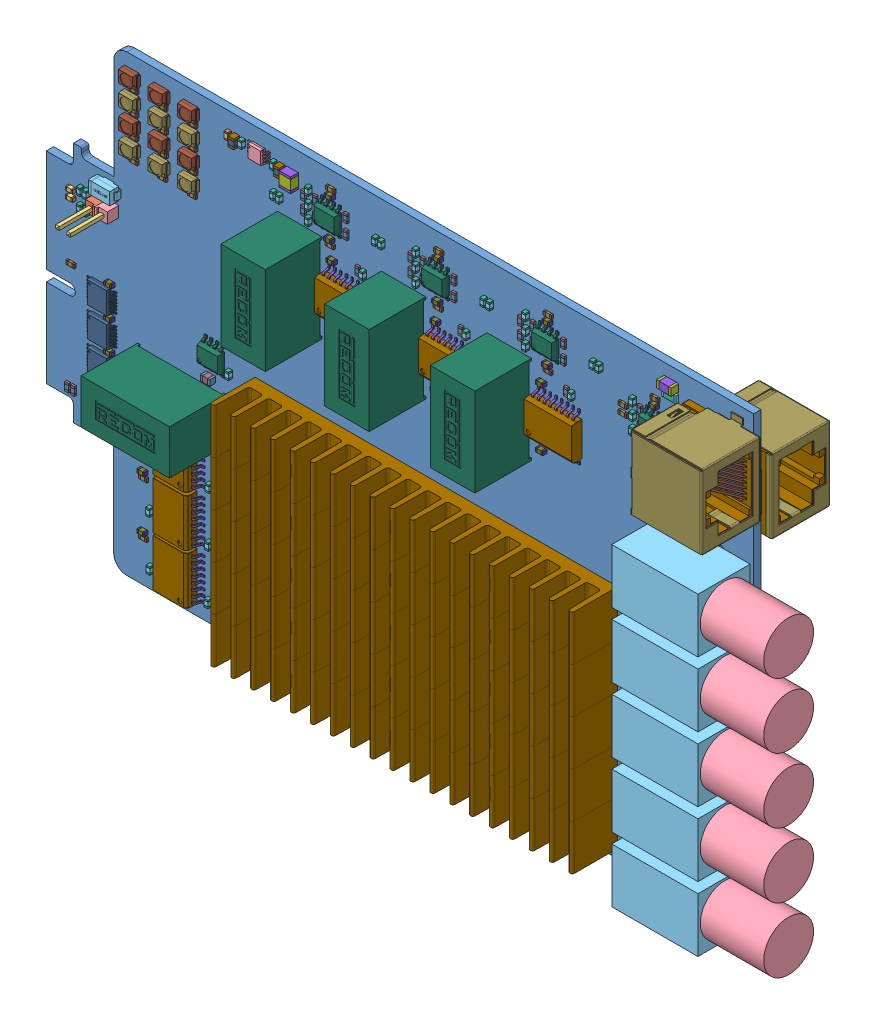
SolidWorks assembly 1166V10, configuration Standard. Lengths in mm. (continued)
Components (placement in the parent): (continued)
- 1166V10.step-1: 1166V10.step [Standard] at origin size (170.01 100 28.53) (continued)
  - IC401.step-1: IC401.step [Standard] at origin size (10.5 10.6 2.6) (continued)
    - SOIC-16-300.step-1: SOIC-16-300.step [Standard] at (66.9509 76.5501 -3.022) x (1 0 0) z (0 1 0) size (10.5 2.6 10.6) (continued)
      - User_Library-SOIC-16-300_pin_SOIC_SO-300_1.step-2: User_Library-SOIC-16-300_pin_SOIC_SO-300_1.step [Standard] at (1.905 0 -3.8) x (-1 0 0) z (0 0 -1) size (0.4 1.55 1.5)
      - User_Library-SOIC-16-300_pin_SOIC_SO-300_1.step-3: User_Library-SOIC-16-300_pin_SOIC_SO-300_1.step [Standard] at (4.445 0 -3.8) x (-1 0 0) z (0 0 -1) size (0.4 1.55 1.5)
      - User_Library-SOIC-16-300_SOIC_300_SOIC_10.5X7.6_1.step-1: User_Library-SOIC-16-300_SOIC_300_SOIC_10.5X7.6_1.step [Standard] at origin size (10.5 2.35 7.6)
      - User_Library-SOIC-16-300_pin_SOIC_SO-300_1.step-4: User_Library-SOIC-16-300_pin_SOIC_SO-300_1.step [Standard] at (-3.175 0 -3.8) x (-1 0 0) z (0 0 -1) size (0.4 1.55 1.5)
      - User_Library-SOIC-16-300_pin_SOIC_SO-300_1.step-5: User_Library-SOIC-16-300_pin_SOIC_SO-300_1.step [Standard] at (-3.175 0 3.8) size (0.4 1.55 1.5)
      - User_Library-SOIC-16-300_pin_SOIC_SO-300_1.step-6: User_Library-SOIC-16-300_pin_SOIC_SO-300_1.step [Standard] at (1.905 0 3.8) size (0.4 1.55 1.5)
      - User_Library-SOIC-16-300_pin_SOIC_SO-300_1.step-7: User_Library-SOIC-16-300_pin_SOIC_SO-300_1.step [Standard] at (-1.905 0 3.8) size (0.4 1.55 1.5)
      - User_Library-SOIC-16-300_pin_SOIC_SO-300_1.step-8: User_Library-SOIC-16-300_pin_SOIC_SO-300_1.step [Standard] at (0.635 0 3.8) size (0.4 1.55 1.5)
      - User_Library-SOIC-16-300_pin_SOIC_SO-300_1.step-9: User_Library-SOIC-16-300_pin_SOIC_SO-300_1.step [Standard] at (3.175 0 3.8) size (0.4 1.55 1.5)
      - User_Library-SOIC-16-300_pin_SOIC_SO-300_1.step-10: User_Library-SOIC-16-300_pin_SOIC_SO-300_1.step [Standard] at (4.445 0 3.8) size (0.4 1.55 1.5)
      - User_Library-SOIC-16-300_pin_SOIC_SO-300_1.step-11: User_Library-SOIC-16-300_pin_SOIC_SO-300_1.step [Standard] at (-0.635 0 -3.8) x (-1 0 0) z (0 0 -1) size (0.4 1.55 1.5)
      - User_Library-SOIC-16-300_pin_SOIC_SO-300_1.step-12: User_Library-SOIC-16-300_pin_SOIC_SO-300_1.step [Standard] at (-4.445 0 3.8) size (0.4 1.55 1.5)
      - User_Library-SOIC-16-300_pin_SOIC_SO-300_1.step-13: User_Library-SOIC-16-300_pin_SOIC_SO-300_1.step [Standard] at (3.175 0 -3.8) x (-1 0 0) z (0 0 -1) size (0.4 1.55 1.5)
      - User_Library-SOIC-16-300_pin_SOIC_SO-300_1.step-14: User_Library-SOIC-16-300_pin_SOIC_SO-300_1.step [Standard] at (-0.635 0 3.8) size (0.4 1.55 1.5)
      - User_Library-SOIC-16-300_pin_SOIC_SO-300_1.step-15: User_Library-SOIC-16-300_pin_SOIC_SO-300_1.step [Standard] at (-4.445 0 -3.8) x (-1 0 0) z (0 0 -1) size (0.4 1.55 1.5)
      - User_Library-SOIC-16-300_pin_SOIC_SO-300_1.step-16: User_Library-SOIC-16-300_pin_SOIC_SO-300_1.step [Standard] at (-1.905 0 -3.8) x (-1 0 0) z (0 0 -1) size (0.4 1.55 1.5)
  - IC301.step-1: IC301.step [Standard] at origin size (10.5 10.6 2.6)
    - SOIC-16-300.step-1: SOIC-16-300.step [Standard] at (89.8509 76.5501 -3.022) x (1 0 0) z (0 1 0) size (10.5 2.6 10.6)
      - User_Library-SOIC-16-300_pin_SOIC_SO-300_1.step-1: User_Library-SOIC-16-300_pin_SOIC_SO-300_1.step [Standard] at (0.635 0 -3.8) x (-1 0 0) z (0 0 -1) size (0.4 1.55 1.5)
      - User_Library-SOIC-16-300_pin_SOIC_SO-300_1.step-2: User_Library-SOIC-16-300_pin_SOIC_SO-300_1.step [Standard] at (1.905 0 -3.8) x (-1 0 0) z (0 0 -1) size (0.4 1.55 1.5)
      - User_Library-SOIC-16-300_pin_SOIC_SO-300_1.step-3: User_Library-SOIC-16-300_pin_SOIC_SO-300_1.step [Standard] at (4.445 0 -3.8) x (-1 0 0) z (0 0 -1) size (0.4 1.55 1.5)
      - User_Library-SOIC-16-300_SOIC_300_SOIC_10.5X7.6_1.step-1: User_Library-SOIC-16-300_SOIC_300_SOIC_10.5X7.6_1.step [Standard] at origin size (10.5 2.35 7.6)
      - User_Library-SOIC-16-300_pin_SOIC_SO-300_1.step-4: User_Library-SOIC-16-300_pin_SOIC_SO-300_1.step [Standard] at (-3.175 0 -3.8) x (-1 0 0) z (0 0 -1) size (0.4 1.55 1.5)
      - User_Library-SOIC-16-300_pin_SOIC_SO-300_1.step-5: User_Library-SOIC-16-300_pin_SOIC_SO-300_1.step [Standard] at (-3.175 0 3.8) size (0.4 1.55 1.5)
      - User_Library-SOIC-16-300_pin_SOIC_SO-300_1.step-6: User_Library-SOIC-16-300_pin_SOIC_SO-300_1.step [Standard] at (1.905 0 3.8) size (0.4 1.55 1.5)
      - User_Library-SOIC-16-300_pin_SOIC_SO-300_1.step-7: User_Library-SOIC-16-300_pin_SOIC_SO-300_1.step [Standard] at (-1.905 0 3.8) size (0.4 1.55 1.5)
      - User_Library-SOIC-16-300_pin_SOIC_SO-300_1.step-8: User_Library-SOIC-16-300_pin_SOIC_SO-300_1.step [Standard] at (0.635 0 3.8) size (0.4 1.55 1.5)
      - User_Library-SOIC-16-300_pin_SOIC_SO-300_1.step-9: User_Library-SOIC-16-300_pin_SOIC_SO-300_1.step [Standard] at (3.175 0 3.8) size (0.4 1.55 1.5)
      - User_Library-SOIC-16-300_pin_SOIC_SO-300_1.step-10: User_Library-SOIC-16-300_pin_SOIC_SO-300_1.step [Standard] at (4.445 0 3.8) size (0.4 1.55 1.5)
      - User_Library-SOIC-16-300_pin_SOIC_SO-300_1.step-11: User_Library-SOIC-16-300_pin_SOIC_SO-300_1.step [Standard] at (-0.635 0 -3.8) x (-1 0 0) z (0 0 -1) size (0.4 1.55 1.5)
      - User_Library-SOIC-16-300_pin_SOIC_SO-300_1.step-12: User_Library-SOIC-16-300_pin_SOIC_SO-300_1.step [Standard] at (-4.445 0 3.8) size (0.4 1.55 1.5)
      - User_Library-SOIC-16-300_pin_SOIC_SO-300_1.step-13: User_Library-SOIC-16-300_pin_SOIC_SO-300_1.step [Standard] at (3.175 0 -3.8) x (-1 0 0) z (0 0 -1) size (0.4 1.55 1.5)
      - User_Library-SOIC-16-300_pin_SOIC_SO-300_1.step-14: User_Library-SOIC-16-300_pin_SOIC_SO-300_1.step [Standard] at (-0.635 0 3.8) size (0.4 1.55 1.5)
      - User_Library-SOIC-16-300_pin_SOIC_SO-300_1.step-15: User_Library-SOIC-16-300_pin_SOIC_SO-300_1.step [Standard] at (-4.445 0 -3.8) x (-1 0 0) z (0 0 -1) size (0.4 1.55 1.5)
      - User_Library-SOIC-16-300_pin_SOIC_SO-300_1.step-16: User_Library-SOIC-16-300_pin_SOIC_SO-300_1.step [Standard] at (-1.905 0 -3.8) x (-1 0 0) z (0 0 -1) size (0.4 1.55 1.5)
  - IC201.step-1: IC201.step [Standard] at origin size (10.5 10.6 2.6)
    - SOIC-16-300.step-1: SOIC-16-300.step [Standard] at (113.1509 76.5501 -3.022) x (1 0 0) z (0 1 0) size (10.5 2.6 10.6)
      - User_Library-SOIC-16-300_pin_SOIC_SO-300_1.step-1: User_Library-SOIC-16-300_pin_SOIC_SO-300_1.step [Standard] at (0.635 0 -3.8) x (-1 0 0) z (0 0 -1) size (0.4 1.55 1.5)
      - User_Library-SOIC-16-300_pin_SOIC_SO-300_1.step-2: User_Library-SOIC-16-300_pin_SOIC_SO-300_1.step [Standard] at (1.905 0 -3.8) x (-1 0 0) z (0 0 -1) size (0.4 1.55 1.5)
      - User_Library-SOIC-16-300_pin_SOIC_SO-300_1.step-3: User_Library-SOIC-16-300_pin_SOIC_SO-300_1.step [Standard] at (4.445 0 -3.8) x (-1 0 0) z (0 0 -1) size (0.4 1.55 1.5)
      - User_Library-SOIC-16-300_SOIC_300_SOIC_10.5X7.6_1.step-1: User_Library-SOIC-16-300_SOIC_300_SOIC_10.5X7.6_1.step [Standard] at origin size (10.5 2.35 7.6)
      - User_Library-SOIC-16-300_pin_SOIC_SO-300_1.step-4: User_Library-SOIC-16-300_pin_SOIC_SO-300_1.step [Standard] at (-3.175 0 -3.8) x (-1 0 0) z (0 0 -1) size (0.4 1.55 1.5)
      - User_Library-SOIC-16-300_pin_SOIC_SO-300_1.step-5: User_Library-SOIC-16-300_pin_SOIC_SO-300_1.step [Standard] at (-3.175 0 3.8) size (0.4 1.55 1.5)
      - User_Library-SOIC-16-300_pin_SOIC_SO-300_1.step-6: User_Library-SOIC-16-300_pin_SOIC_SO-300_1.step [Standard] at (1.905 0 3.8) size (0.4 1.55 1.5)
      - User_Library-SOIC-16-300_pin_SOIC_SO-300_1.step-7: User_Library-SOIC-16-300_pin_SOIC_SO-300_1.step [Standard] at (-1.905 0 3.8) size (0.4 1.55 1.5)
      - User_Library-SOIC-16-300_pin_SOIC_SO-300_1.step-8: User_Library-SOIC-16-300_pin_SOIC_SO-300_1.step [Standard] at (0.635 0 3.8) size (0.4 1.55 1.5)
      - User_Library-SOIC-16-300_pin_SOIC_SO-300_1.step-9: User_Library-SOIC-16-300_pin_SOIC_SO-300_1.step [Standard] at (3.175 0 3.8) size (0.4 1.55 1.5)
      - User_Library-SOIC-16-300_pin_SOIC_SO-300_1.step-10: User_Library-SOIC-16-300_pin_SOIC_SO-300_1.step [Standard] at (4.445 0 3.8) size (0.4 1.55 1.5)
      - User_Library-SOIC-16-300_pin_SOIC_SO-300_1.step-11: User_Library-SOIC-16-300_pin_SOIC_SO-300_1.step [Standard] at (-0.635 0 -3.8) x (-1 0 0) z (0 0 -1) size (0.4 1.55 1.5)
      - User_Library-SOIC-16-300_pin_SOIC_SO-300_1.step-12: User_Library-SOIC-16-300_pin_SOIC_SO-300_1.step [Standard] at (-4.445 0 3.8) size (0.4 1.55 1.5)
      - User_Library-SOIC-16-300_pin_SOIC_SO-300_1.step-13: User_Library-SOIC-16-300_pin_SOIC_SO-300_1.step [Standard] at (3.175 0 -3.8) x (-1 0 0) z (0 0 -1) size (0.4 1.55 1.5)
      - User_Library-SOIC-16-300_pin_SOIC_SO-300_1.step-14: User_Library-SOIC-16-300_pin_SOIC_SO-300_1.step [Standard] at (-0.635 0 3.8) size (0.4 1.55 1.5)
      - User_Library-SOIC-16-300_pin_SOIC_SO-300_1.step-15: User_Library-SOIC-16-300_pin_SOIC_SO-300_1.step [Standard] at (-4.445 0 -3.8) x (-1 0 0) z (0 0 -1) size (0.4 1.55 1.5)
      - User_Library-SOIC-16-300_pin_SOIC_SO-300_1.step-16: User_Library-SOIC-16-300_pin_SOIC_SO-300_1.step [Standard] at (-1.905 0 -3.8) x (-1 0 0) z (0 0 -1) size (0.4 1.55 1.5)
  - C422.step-1: C422.step [Standard] at origin size (1.6 0.82 0.9)
    - 6547664352.step-1: 6547664352.step [Standard] at (64.25 65.8 -2.522) size (0.9 0.82 0.9)
      - Extruded-9.step-1: Extruded-9.step [Standard] at origin size (0.9 0.82 0.9)
    - 6547664912.step-1: 6547664912.step [Standard] at (64.875 65.8 -2.522) size (0.35 0.82 0.9)
      - Extruded-10.step-1: Extruded-10.step [Standard] at origin size (0.35 0.82 0.9)
    - 6547664912.step-2: 6547664912.step [Standard] at (63.625 65.8 -2.522) size (0.35 0.82 0.9)
      - Extruded-10.step-1: Extruded-10.step [Standard] at origin size (0.35 0.82 0.9)
  - C421.step-1: C421.step [Standard] at origin size (3.2 1.6 1.7)
    - 6547444720.step-1: 6547444720.step [Standard] at (65.7 67.6 -3.322) size (0.5 1.6 1.7)
      - Extruded-22.step-1: Extruded-22.step [Standard] at origin size (0.5 1.6 1.7)
    - 6547444720.step-2: 6547444720.step [Standard] at (63 67.6 -3.322) size (0.5 1.6 1.7)
      - Extruded-22.step-1: Extruded-22.step [Standard] at origin size (0.5 1.6 1.7)
    - 6547445040.step-1: 6547445040.step [Standard] at (64.35 67.6 -3.322) size (2.2 1.6 1.7)
      - Extruded-23.step-1: Extruded-23.step [Standard] at origin size (2.2 1.6 1.7)
  - C420.step-1: C420.step [Standard] at origin size (3.2 1.6 1.7)
    - 6547444720.step-1: 6547444720.step [Standard] at (65.7 69.7 -3.322) size (0.5 1.6 1.7)
      - Extruded-22.step-1: Extruded-22.step [Standard] at origin size (0.5 1.6 1.7)
    - 6547444720.step-2: 6547444720.step [Standard] at (63 69.7 -3.322) size (0.5 1.6 1.7)
      - Extruded-22.step-1: Extruded-22.step [Standard] at origin size (0.5 1.6 1.7)
    - 6547445040.step-1: 6547445040.step [Standard] at (64.35 69.7 -3.322) size (2.2 1.6 1.7)
      - Extruded-23.step-1: Extruded-23.step [Standard] at origin size (2.2 1.6 1.7)
  - C419.step-1: C419.step [Standard] at origin size (1.6 0.82 0.9)
    - 6547664352.step-1: 6547664352.step [Standard] at (68.25 70 -2.522) size (0.9 0.82 0.9)
      - Extruded-9.step-1: Extruded-9.step [Standard] at origin size (0.9 0.82 0.9)
    - 6547664912.step-1: 6547664912.step [Standard] at (68.875 70 -2.522) size (0.35 0.82 0.9)
      - Extruded-10.step-1: Extruded-10.step [Standard] at origin size (0.35 0.82 0.9)
    - 6547664912.step-2: 6547664912.step [Standard] at (67.625 70 -2.522) size (0.35 0.82 0.9)
      - Extruded-10.step-1: Extruded-10.step [Standard] at origin size (0.35 0.82 0.9)
  - C418.step-1: C418.step [Standard] at origin size (1.6 0.82 0.9)
    - 6547664352.step-1: 6547664352.step [Standard] at (71.15 70 -2.522) size (0.9 0.82 0.9)
      - Extruded-9.step-1: Extruded-9.step [Standard] at origin size (0.9 0.82 0.9)
    - 6547664912.step-1: 6547664912.step [Standard] at (70.525 70 -2.522) size (0.35 0.82 0.9)
      - Extruded-10.step-1: Extruded-10.step [Standard] at origin size (0.35 0.82 0.9)
    - 6547664912.step-2: 6547664912.step [Standard] at (71.775 70 -2.522) size (0.35 0.82 0.9)
      - Extruded-10.step-1: Extruded-10.step [Standard] at origin size (0.35 0.82 0.9)
  - C417.step-1: C417.step [Standard] at origin size (1.6 0.82 0.9)
    - 6547664352.step-1: 6547664352.step [Standard] at (71.15 68.7 -2.522) size (0.9 0.82 0.9)
      - Extruded-9.step-1: Extruded-9.step [Standard] at origin size (0.9 0.82 0.9)
    - 6547664912.step-1: 6547664912.step [Standard] at (70.525 68.7 -2.522) size (0.35 0.82 0.9)
      - Extruded-10.step-1: Extruded-10.step [Standard] at origin size (0.35 0.82 0.9)
    - 6547664912.step-2: 6547664912.step [Standard] at (71.775 68.7 -2.522) size (0.35 0.82 0.9)
      - Extruded-10.step-1: Extruded-10.step [Standard] at origin size (0.35 0.82 0.9)
  - C415.step-1: C415.step [Standard] at origin size (3.2 1.6 1.7)
    - 6547444720.step-1: 6547444720.step [Standard] at (65.8 83.4 -3.322) size (0.5 1.6 1.7)
      - Extruded-22.step-1: Extruded-22.step [Standard] at origin size (0.5 1.6 1.7)
    - 6547444720.step-2: 6547444720.step [Standard] at (63.1 83.4 -3.322) size (0.5 1.6 1.7)
      - Extruded-22.step-1: Extruded-22.step [Standard] at origin size (0.5 1.6 1.7)
    - 6547445040.step-1: 6547445040.step [Standard] at (64.45 83.4 -3.322) size (2.2 1.6 1.7)
      - Extruded-23.step-1: Extruded-23.step [Standard] at origin size (2.2 1.6 1.7)
  - C414.step-1: C414.step [Standard] at origin size (3.2 1.6 1.7)
    - 6547444720.step-1: 6547444720.step [Standard] at (65.8 85.5 -3.322) size (0.5 1.6 1.7)
      - Extruded-22.step-1: Extruded-22.step [Standard] at origin size (0.5 1.6 1.7)
    - 6547444720.step-2: 6547444720.step [Standard] at (63.1 85.5 -3.322) size (0.5 1.6 1.7)
      - Extruded-22.step-1: Extruded-22.step [Standard] at origin size (0.5 1.6 1.7)
    - 6547445040.step-1: 6547445040.step [Standard] at (64.45 85.5 -3.322) size (2.2 1.6 1.7)
      - Extruded-23.step-1: Extruded-23.step [Standard] at origin size (2.2 1.6 1.7)
  - C413.step-1: C413.step [Standard] at origin size (1.6 0.82 0.9)
    - 6547664352.step-1: 6547664352.step [Standard] at (70.55 83 -2.522) size (0.9 0.82 0.9)
      - Extruded-9.step-1: Extruded-9.step [Standard] at origin size (0.9 0.82 0.9)
    - 6547664912.step-1: 6547664912.step [Standard] at (71.175 83 -2.522) size (0.35 0.82 0.9)
      - Extruded-10.step-1: Extruded-10.step [Standard] at origin size (0.35 0.82 0.9)
    - 6547664912.step-2: 6547664912.step [Standard] at (69.925 83 -2.522) size (0.35 0.82 0.9)
      - Extruded-10.step-1: Extruded-10.step [Standard] at origin size (0.35 0.82 0.9)
  - C322.step-1: C322.step [Standard] at origin size (1.6 0.82 0.9)
    - 6547664352.step-1: 6547664352.step [Standard] at (87.15 65.5 -2.522) size (0.9 0.82 0.9)
      - Extruded-9.step-1: Extruded-9.step [Standard] at origin size (0.9 0.82 0.9)
    - 6547664912.step-1: 6547664912.step [Standard] at (87.775 65.5 -2.522) size (0.35 0.82 0.9)
      - Extruded-10.step-1: Extruded-10.step [Standard] at origin size (0.35 0.82 0.9)
    - 6547664912.step-2: 6547664912.step [Standard] at (86.525 65.5 -2.522) size (0.35 0.82 0.9)
      - Extruded-10.step-1: Extruded-10.step [Standard] at origin size (0.35 0.82 0.9)
  - C321.step-1: C321.step [Standard] at origin size (3.2 1.6 1.7)
    - 6547444720.step-1: 6547444720.step [Standard] at (88.5 67.6 -3.322) size (0.5 1.6 1.7)
      - Extruded-22.step-1: Extruded-22.step [Standard] at origin size (0.5 1.6 1.7)
    - 6547444720.step-2: 6547444720.step [Standard] at (85.8 67.6 -3.322) size (0.5 1.6 1.7)
      - Extruded-22.step-1: Extruded-22.step [Standard] at origin size (0.5 1.6 1.7)
    - 6547445040.step-1: 6547445040.step [Standard] at (87.15 67.6 -3.322) size (2.2 1.6 1.7)
      - Extruded-23.step-1: Extruded-23.step [Standard] at origin size (2.2 1.6 1.7)
  - C320.step-1: C320.step [Standard] at origin size (3.2 1.6 1.7)
    - 6547444720.step-1: 6547444720.step [Standard] at (88.5 69.7 -3.322) size (0.5 1.6 1.7)
      - Extruded-22.step-1: Extruded-22.step [Standard] at origin size (0.5 1.6 1.7)
    - 6547444720.step-2: 6547444720.step [Standard] at (85.8 69.7 -3.322) size (0.5 1.6 1.7)
      - Extruded-22.step-1: Extruded-22.step [Standard] at origin size (0.5 1.6 1.7)
    - 6547445040.step-1: 6547445040.step [Standard] at (87.15 69.7 -3.322) size (2.2 1.6 1.7)
      - Extruded-23.step-1: Extruded-23.step [Standard] at origin size (2.2 1.6 1.7)
  - C319.step-1: C319.step [Standard] at origin size (1.6 0.82 0.9)
    - 6547664352.step-1: 6547664352.step [Standard] at (91.15 70 -2.522) size (0.9 0.82 0.9)
      - Extruded-9.step-1: Extruded-9.step [Standard] at origin size (0.9 0.82 0.9)
    - 6547664912.step-1: 6547664912.step [Standard] at (91.775 70 -2.522) size (0.35 0.82 0.9)
      - Extruded-10.step-1: Extruded-10.step [Standard] at origin size (0.35 0.82 0.9)
    - 6547664912.step-2: 6547664912.step [Standard] at (90.525 70 -2.522) size (0.35 0.82 0.9)
      - Extruded-10.step-1: Extruded-10.step [Standard] at origin size (0.35 0.82 0.9)
  - C318.step-1: C318.step [Standard] at origin size (1.6 0.82 0.9)
    - 6547664352.step-1: 6547664352.step [Standard] at (94.05 70 -2.522) size (0.9 0.82 0.9)
      - Extruded-9.step-1: Extruded-9.step [Standard] at origin size (0.9 0.82 0.9)
    - 6547664912.step-1: 6547664912.step [Standard] at (93.425 70 -2.522) size (0.35 0.82 0.9)
      - Extruded-10.step-1: Extruded-10.step [Standard] at origin size (0.35 0.82 0.9)
    - 6547664912.step-2: 6547664912.step [Standard] at (94.675 70 -2.522) size (0.35 0.82 0.9)
      - Extruded-10.step-1: Extruded-10.step [Standard] at origin size (0.35 0.82 0.9)
  - C317.step-1: C317.step [Standard] at origin size (1.6 0.82 0.9)
    - 6547664352.step-1: 6547664352.step [Standard] at (94.05 68.7 -2.522) size (0.9 0.82 0.9)
      - Extruded-9.step-1: Extruded-9.step [Standard] at origin size (0.9 0.82 0.9)
    - 6547664912.step-1: 6547664912.step [Standard] at (93.425 68.7 -2.522) size (0.35 0.82 0.9)
      - Extruded-10.step-1: Extruded-10.step [Standard] at origin size (0.35 0.82 0.9)
    - 6547664912.step-2: 6547664912.step [Standard] at (94.675 68.7 -2.522) size (0.35 0.82 0.9)
      - Extruded-10.step-1: Extruded-10.step [Standard] at origin size (0.35 0.82 0.9)
  - C315.step-1: C315.step [Standard] at origin size (3.2 1.6 1.7)
    - 6547444720.step-1: 6547444720.step [Standard] at (88.7 83.4 -3.322) size (0.5 1.6 1.7)
      - Extruded-22.step-1: Extruded-22.step [Standard] at origin size (0.5 1.6 1.7)
    - 6547444720.step-2: 6547444720.step [Standard] at (86 83.4 -3.322) size (0.5 1.6 1.7)
      - Extruded-22.step-1: Extruded-22.step [Standard] at origin size (0.5 1.6 1.7)
    - 6547445040.step-1: 6547445040.step [Standard] at (87.35 83.4 -3.322) size (2.2 1.6 1.7)
      - Extruded-23.step-1: Extruded-23.step [Standard] at origin size (2.2 1.6 1.7)
  - C314.step-1: C314.step [Standard] at origin size (3.2 1.6 1.7)
    - 6547444720.step-1: 6547444720.step [Standard] at (88.7 85.5 -3.322) size (0.5 1.6 1.7)
      - Extruded-22.step-1: Extruded-22.step [Standard] at origin size (0.5 1.6 1.7)
    - 6547444720.step-2: 6547444720.step [Standard] at (86 85.5 -3.322) size (0.5 1.6 1.7)
      - Extruded-22.step-1: Extruded-22.step [Standard] at origin size (0.5 1.6 1.7)
    - 6547445040.step-1: 6547445040.step [Standard] at (87.35 85.5 -3.322) size (2.2 1.6 1.7)
      - Extruded-23.step-1: Extruded-23.step [Standard] at origin size (2.2 1.6 1.7)
  - C313.step-1: C313.step [Standard] at origin size (1.6 0.82 0.9)
    - 6547664352.step-1: 6547664352.step [Standard] at (93.45 83 -2.522) size (0.9 0.82 0.9)
      - Extruded-9.step-1: Extruded-9.step [Standard] at origin size (0.9 0.82 0.9)
    - 6547664912.step-1: 6547664912.step [Standard] at (94.075 83 -2.522) size (0.35 0.82 0.9)
      - Extruded-10.step-1: Extruded-10.step [Standard] at origin size (0.35 0.82 0.9)
    - 6547664912.step-2: 6547664912.step [Standard] at (92.825 83 -2.522) size (0.35 0.82 0.9)
      - Extruded-10.step-1: Extruded-10.step [Standard] at origin size (0.35 0.82 0.9)
  - C222.step-1: C222.step [Standard] at origin size (1.6 0.82 0.9)
    - 6547664352.step-1: 6547664352.step [Standard] at (110.65 65.6 -2.522) size (0.9 0.82 0.9)
      - Extruded-9.step-1: Extruded-9.step [Standard] at origin size (0.9 0.82 0.9)
    - 6547664912.step-1: 6547664912.step [Standard] at (111.275 65.6 -2.522) size (0.35 0.82 0.9)
      - Extruded-10.step-1: Extruded-10.step [Standard] at origin size (0.35 0.82 0.9)
    - 6547664912.step-2: 6547664912.step [Standard] at (110.025 65.6 -2.522) size (0.35 0.82 0.9)
      - Extruded-10.step-1: Extruded-10.step [Standard] at origin size (0.35 0.82 0.9)
  - C221.step-1: C221.step [Standard] at origin size (3.2 1.6 1.7)
    - 6547444720.step-1: 6547444720.step [Standard] at (111.9 69.6 -3.322) size (0.5 1.6 1.7)
      - Extruded-22.step-1: Extruded-22.step [Standard] at origin size (0.5 1.6 1.7)
    - 6547444720.step-2: 6547444720.step [Standard] at (109.2 69.6 -3.322) size (0.5 1.6 1.7)
      - Extruded-22.step-1: Extruded-22.step [Standard] at origin size (0.5 1.6 1.7)
    - 6547445040.step-1: 6547445040.step [Standard] at (110.55 69.6 -3.322) size (2.2 1.6 1.7)
      - Extruded-23.step-1: Extruded-23.step [Standard] at origin size (2.2 1.6 1.7)
  - C220.step-1: C220.step [Standard] at origin size (3.2 1.6 1.7)
    - 6547444720.step-1: 6547444720.step [Standard] at (111.9 67.5 -3.322) size (0.5 1.6 1.7)
      - Extruded-22.step-1: Extruded-22.step [Standard] at origin size (0.5 1.6 1.7)
    - 6547444720.step-2: 6547444720.step [Standard] at (109.2 67.5 -3.322) size (0.5 1.6 1.7)
      - Extruded-22.step-1: Extruded-22.step [Standard] at origin size (0.5 1.6 1.7)
    - 6547445040.step-1: 6547445040.step [Standard] at (110.55 67.5 -3.322) size (2.2 1.6 1.7)
      - Extruded-23.step-1: Extruded-23.step [Standard] at origin size (2.2 1.6 1.7)
  - C219.step-1: C219.step [Standard] at origin size (1.6 0.82 0.9)
    - 6547664352.step-1: 6547664352.step [Standard] at (114.45 69.9 -2.522) size (0.9 0.82 0.9)
      - Extruded-9.step-1: Extruded-9.step [Standard] at origin size (0.9 0.82 0.9)
    - 6547664912.step-1: 6547664912.step [Standard] at (115.075 69.9 -2.522) size (0.35 0.82 0.9)
      - Extruded-10.step-1: Extruded-10.step [Standard] at origin size (0.35 0.82 0.9)
    - 6547664912.step-2: 6547664912.step [Standard] at (113.825 69.9 -2.522) size (0.35 0.82 0.9)
      - Extruded-10.step-1: Extruded-10.step [Standard] at origin size (0.35 0.82 0.9)
  - C218.step-1: C218.step [Standard] at origin size (1.6 0.82 0.9)
    - 6547664352.step-1: 6547664352.step [Standard] at (117.35 69.9 -2.522) size (0.9 0.82 0.9)
      - Extruded-9.step-1: Extruded-9.step [Standard] at origin size (0.9 0.82 0.9)
    - 6547664912.step-1: 6547664912.step [Standard] at (116.725 69.9 -2.522) size (0.35 0.82 0.9)
      - Extruded-10.step-1: Extruded-10.step [Standard] at origin size (0.35 0.82 0.9)
    - 6547664912.step-2: 6547664912.step [Standard] at (117.975 69.9 -2.522) size (0.35 0.82 0.9)
      - Extruded-10.step-1: Extruded-10.step [Standard] at origin size (0.35 0.82 0.9)
  - C217.step-1: C217.step [Standard] at origin size (1.6 0.82 0.9)
    - 6547664352.step-1: 6547664352.step [Standard] at (117.35 68.6 -2.522) size (0.9 0.82 0.9)
      - Extruded-9.step-1: Extruded-9.step [Standard] at origin size (0.9 0.82 0.9)
    - 6547664912.step-1: 6547664912.step [Standard] at (116.725 68.6 -2.522) size (0.35 0.82 0.9)
      - Extruded-10.step-1: Extruded-10.step [Standard] at origin size (0.35 0.82 0.9)
    - 6547664912.step-2: 6547664912.step [Standard] at (117.975 68.6 -2.522) size (0.35 0.82 0.9)
      - Extruded-10.step-1: Extruded-10.step [Standard] at origin size (0.35 0.82 0.9)
  - C215.step-1: C215.step [Standard] at origin size (3.2 1.6 1.7)
    - 6547444720.step-1: 6547444720.step [Standard] at (111.9 83.4 -3.322) size (0.5 1.6 1.7)
      - Extruded-22.step-1: Extruded-22.step [Standard] at origin size (0.5 1.6 1.7)
    - 6547444720.step-2: 6547444720.step [Standard] at (109.2 83.4 -3.322) size (0.5 1.6 1.7)
      - Extruded-22.step-1: Extruded-22.step [Standard] at origin size (0.5 1.6 1.7)
    - 6547445040.step-1: 6547445040.step [Standard] at (110.55 83.4 -3.322) size (2.2 1.6 1.7)
      - Extruded-23.step-1: Extruded-23.step [Standard] at origin size (2.2 1.6 1.7)
  - C214.step-1: C214.step [Standard] at origin size (3.2 1.6 1.7)
    - 6547444720.step-1: 6547444720.step [Standard] at (111.9 85.5 -3.322) size (0.5 1.6 1.7)
      - Extruded-22.step-1: Extruded-22.step [Standard] at origin size (0.5 1.6 1.7)
    - 6547444720.step-2: 6547444720.step [Standard] at (109.2 85.5 -3.322) size (0.5 1.6 1.7)
      - Extruded-22.step-1: Extruded-22.step [Standard] at origin size (0.5 1.6 1.7)
    - 6547445040.step-1: 6547445040.step [Standard] at (110.55 85.5 -3.322) size (2.2 1.6 1.7)
      - Extruded-23.step-1: Extruded-23.step [Standard] at origin size (2.2 1.6 1.7)
  - C213.step-1: C213.step [Standard] at origin size (1.6 0.82 0.9)
    - 6547664352.step-1: 6547664352.step [Standard] at (116.75 83 -2.522) size (0.9 0.82 0.9)
      - Extruded-9.step-1: Extruded-9.step [Standard] at origin size (0.9 0.82 0.9)
    - 6547664912.step-1: 6547664912.step [Standard] at (117.375 83 -2.522) size (0.35 0.82 0.9)
      - Extruded-10.step-1: Extruded-10.step [Standard] at origin size (0.35 0.82 0.9)
    - 6547664912.step-2: 6547664912.step [Standard] at (116.125 83 -2.522) size (0.35 0.82 0.9)
      - Extruded-10.step-1: Extruded-10.step [Standard] at origin size (0.35 0.82 0.9)
  - J103.step-1: J103.step [Standard] at origin size (16.3 18.8 14.7)
    - 634008149821.step-1: 634008149821.step [Standard] at (150.1251 88.6499 6.78) x (0 1 0) z (0 0 1) size (18.8 16.3 14.7)
      - 634008149821_Housing.step-1: 634008149821_Housing.step [Standard] at origin size (15.9 15.05 14.45)
      - 634008149821_Housing2.step-1: 634008149821_Housing2.step [Standard] at (0 2.025 -5.6) x (-1 0 0) z (0 0 1) size (9.9 7.7 1.95)
      - 634008149821_Pin.step-1: 634008149821_Pin.step [Standard] at (3.57 -0.6678 -5.975) size (0.45 14.79 5.55)
      - 634008149821_Pin.step-2: 634008149821_Pin.step [Standard] at (2.55 -0.6678 -5.975) size (0.45 14.79 5.55)
      - 634008149821_Pin.step-3: 634008149821_Pin.step [Standard] at (1.53 -0.6678 -5.975) size (0.45 14.79 5.55)
      - 634008149821_Pin.step-4: 634008149821_Pin.step [Standard] at (0.51 -0.6678 -5.975) size (0.45 14.79 5.55)
      - 634008149821_Pin.step-5: 634008149821_Pin.step [Standard] at (-0.51 -0.6678 -5.975) size (0.45 14.79 5.55)
      - 634008149821_Pin.step-6: 634008149821_Pin.step [Standard] at (-1.53 -0.6678 -5.975) size (0.45 14.79 5.55)
      - 634008149821_Pin.step-7: 634008149821_Pin.step [Standard] at (-2.55 -0.6678 -5.975) size (0.45 14.79 5.55)
      - 634008149821_Pin.step-8: 634008149821_Pin.step [Standard] at (-3.57 -0.6678 -5.975) size (0.45 14.79 5.55)
      - 634008149821_Shielding.step-1: 634008149821_Shielding.step [Standard] at (0 0.075 0.125) size (18.8 15.7 13.48)
  - J102.step-1: J102.step [Standard] at origin size (16.3 18.8 14.7)
    - 634008149821.step-1: 634008149821.step [Standard] at (150.1001 84.0001 -8.402) x (0 -1 0) z (0 0 -1) size (18.8 16.3 14.7)
      - 634008149821_Housing.step-1: 634008149821_Housing.step [Standard] at origin size (15.9 15.05 14.45)
      - 634008149821_Housing2.step-1: 634008149821_Housing2.step [Standard] at (0 2.025 -5.6) x (-1 0 0) z (0 0 1) size (9.9 7.7 1.95)
      - 634008149821_Pin.step-1: 634008149821_Pin.step [Standard] at (3.57 -0.6678 -5.975) size (0.45 14.79 5.55)
      - 634008149821_Pin.step-2: 634008149821_Pin.step [Standard] at (2.55 -0.6678 -5.975) size (0.45 14.79 5.55)
      - 634008149821_Pin.step-3: 634008149821_Pin.step [Standard] at (1.53 -0.6678 -5.975) size (0.45 14.79 5.55)
      - 634008149821_Pin.step-4: 634008149821_Pin.step [Standard] at (0.51 -0.6678 -5.975) size (0.45 14.79 5.55)
      - 634008149821_Pin.step-5: 634008149821_Pin.step [Standard] at (-0.51 -0.6678 -5.975) size (0.45 14.79 5.55)
      - 634008149821_Pin.step-6: 634008149821_Pin.step [Standard] at (-1.53 -0.6678 -5.975) size (0.45 14.79 5.55)
      - 634008149821_Pin.step-7: 634008149821_Pin.step [Standard] at (-2.55 -0.6678 -5.975) size (0.45 14.79 5.55)
      - 634008149821_Pin.step-8: 634008149821_Pin.step [Standard] at (-3.57 -0.6678 -5.975) size (0.45 14.79 5.55)
      - 634008149821_Shielding.step-1: 634008149821_Shielding.step [Standard] at (0 0.075 0.125) size (18.8 15.7 13.48)
  - R417.step-1: R417.step [Standard] at origin size (0.85 1.85 0.45)
    - 6549605488.step-1: 6549605488.step [Standard] at (40.9 8.95 -2.072) size (0.85 0.95 0.45)
      - Extruded-8.step-1: Extruded-8.step [Standard] at origin size (0.85 0.95 0.45)
    - 6549605008.step-1: 6549605008.step [Standard] at (40.9 8.25 -2.072) size (0.85 0.45 0.45)
      - Extruded-7.step-1: Extruded-7.step [Standard] at origin size (0.85 0.45 0.45)
    - 6549605008.step-2: 6549605008.step [Standard] at (40.9 9.65 -2.072) size (0.85 0.45 0.45)
      - Extruded-7.step-1: Extruded-7.step [Standard] at origin size (0.85 0.45 0.45)
  - R317.step-1: R317.step [Standard] at origin size (0.85 1.85 0.45)
    - 6549605488.step-1: 6549605488.step [Standard] at (40.9 19.95 -2.072) size (0.85 0.95 0.45)
      - Extruded-8.step-1: Extruded-8.step [Standard] at origin size (0.85 0.95 0.45)
    - 6549605008.step-1: 6549605008.step [Standard] at (40.9 19.25 -2.072) size (0.85 0.45 0.45)
      - Extruded-7.step-1: Extruded-7.step [Standard] at origin size (0.85 0.45 0.45)
    - 6549605008.step-2: 6549605008.step [Standard] at (40.9 20.65 -2.072) size (0.85 0.45 0.45)
      - Extruded-7.step-1: Extruded-7.step [Standard] at origin size (0.85 0.45 0.45)
  - R217.step-1: R217.step [Standard] at origin size (0.85 1.85 0.45)
    - 6549605488.step-1: 6549605488.step [Standard] at (40.9 30.95 -2.072) size (0.85 0.95 0.45)
      - Extruded-8.step-1: Extruded-8.step [Standard] at origin size (0.85 0.95 0.45)
    - 6549605008.step-1: 6549605008.step [Standard] at (40.9 30.25 -2.072) size (0.85 0.45 0.45)
      - Extruded-7.step-1: Extruded-7.step [Standard] at origin size (0.85 0.45 0.45)
    - 6549605008.step-2: 6549605008.step [Standard] at (40.9 31.65 -2.072) size (0.85 0.45 0.45)
      - Extruded-7.step-1: Extruded-7.step [Standard] at origin size (0.85 0.45 0.45)
  - R216.step-1: R216.step [Standard] at origin size (0.85 1.85 0.45)
    - 6549605008.step-1: 6549605008.step [Standard] at (104.8 88.75 0) size (0.85 0.45 0.45)
      - Extruded-7.step-1: Extruded-7.step [Standard] at origin size (0.85 0.45 0.45)
    - 6549605008.step-2: 6549605008.step [Standard] at (104.8 90.15 0) size (0.85 0.45 0.45)
      - Extruded-7.step-1: Extruded-7.step [Standard] at origin size (0.85 0.45 0.45)
    - 6549605488.step-1: 6549605488.step [Standard] at (104.8 89.45 0) size (0.85 0.95 0.45)
      - Extruded-8.step-1: Extruded-8.step [Standard] at origin size (0.85 0.95 0.45)
  - R213.step-1: R213.step [Standard] at origin size (0.85 1.85 0.45)
    - 6549605008.step-1: 6549605008.step [Standard] at (104.8 91.65 0) size (0.85 0.45 0.45)
      - Extruded-7.step-1: Extruded-7.step [Standard] at origin size (0.85 0.45 0.45)
    - 6549605008.step-2: 6549605008.step [Standard] at (104.8 93.05 0) size (0.85 0.45 0.45)
      - Extruded-7.step-1: Extruded-7.step [Standard] at origin size (0.85 0.45 0.45)
    - 6549605488.step-1: 6549605488.step [Standard] at (104.8 92.35 0) size (0.85 0.95 0.45)
      - Extruded-8.step-1: Extruded-8.step [Standard] at origin size (0.85 0.95 0.45)
  - IC404.step-1: IC404.step [Standard] at origin size (10.64 4.83 1.7)
    - SOIC-8_Wide.step-1: SOIC-8_Wide.step [Standard] at (29.7001 11.0001 -1.622) x (0 1 0) z (-1 0 0) size (4.83 1.7 10.64)
  - IC304.step-1: IC304.step [Standard] at origin size (10.64 4.83 1.7)
    - SOIC-8_Wide.step-1: SOIC-8_Wide.step [Standard] at (29.7001 22.0001 -1.622) x (0 1 0) z (-1 0 0) size (4.83 1.7 10.64)
  - IC203.step-1: IC203.step [Standard] at origin size (4.83 6.2 1.7)
    - SOIC-8_Narrow.step-1: SOIC-8_Narrow.step [Standard] at (35.2599 51.7146 0) x (-1 0 0) z (0 1 0) size (4.83 1.7 6.2)
  - IC205.step-1: IC205.step [Standard] at origin size (10.64 4.83 1.7)
    - SOIC-8_Wide.step-1: SOIC-8_Wide.step [Standard] at (29.7001 33.1001 -1.622) x (0 1 0) z (-1 0 0) size (4.83 1.7 10.64)
  - CF410.step-1: CF410.step [Standard] at origin size (0.82 1.6 0.9)
    - 6549602528.step-1: 6549602528.step [Standard] at (38.2 10.375 -2.522) size (0.82 0.35 0.9)
      - Extruded-0.step-1: Extruded-0.step [Standard] at origin size (0.82 0.35 0.9)
    - 6549602528.step-2: 6549602528.step [Standard] at (38.2 9.125 -2.522) size (0.82 0.35 0.9)
      - Extruded-0.step-1: Extruded-0.step [Standard] at origin size (0.82 0.35 0.9)
    - 6547668352.step-1: 6547668352.step [Standard] at (38.2 9.75 -2.522) size (0.82 0.9 0.9)
      - Extruded.step-1: Extruded.step [Standard] at origin size (0.82 0.9 0.9)
  - CF409.step-1: CF409.step [Standard] at origin size (0.82 1.6 0.9)
    - 6549602528.step-1: 6549602528.step [Standard] at (36.9 10.375 -2.522) size (0.82 0.35 0.9)
      - Extruded-0.step-1: Extruded-0.step [Standard] at origin size (0.82 0.35 0.9)
    - 6549602528.step-2: 6549602528.step [Standard] at (36.9 9.125 -2.522) size (0.82 0.35 0.9)
      - Extruded-0.step-1: Extruded-0.step [Standard] at origin size (0.82 0.35 0.9)
    - 6547668352.step-1: 6547668352.step [Standard] at (36.9 9.75 -2.522) size (0.82 0.9 0.9)
      - Extruded.step-1: Extruded.step [Standard] at origin size (0.82 0.9 0.9)
  - CF408.step-1: CF408.step [Standard] at origin size (1.6 0.82 0.9)
    - 6547664912.step-1: 6547664912.step [Standard] at (22.275 10.7 -2.522) size (0.35 0.82 0.9)
      - Extruded-10.step-1: Extruded-10.step [Standard] at origin size (0.35 0.82 0.9)
    - 6547664912.step-2: 6547664912.step [Standard] at (21.025 10.7 -2.522) size (0.35 0.82 0.9)
      - Extruded-10.step-1: Extruded-10.step [Standard] at origin size (0.35 0.82 0.9)
    - 6547664352.step-1: 6547664352.step [Standard] at (21.65 10.7 -2.522) size (0.9 0.82 0.9)
      - Extruded-9.step-1: Extruded-9.step [Standard] at origin size (0.9 0.82 0.9)
  - CF407.step-1: CF407.step [Standard] at origin size (1.6 0.82 0.9)
    - 6547664912.step-1: 6547664912.step [Standard] at (22.275 12 -2.522) size (0.35 0.82 0.9)
      - Extruded-10.step-1: Extruded-10.step [Standard] at origin size (0.35 0.82 0.9)
    - 6547664912.step-2: 6547664912.step [Standard] at (21.025 12 -2.522) size (0.35 0.82 0.9)
      - Extruded-10.step-1: Extruded-10.step [Standard] at origin size (0.35 0.82 0.9)
    - 6547664352.step-1: 6547664352.step [Standard] at (21.65 12 -2.522) size (0.9 0.82 0.9)
      - Extruded-9.step-1: Extruded-9.step [Standard] at origin size (0.9 0.82 0.9)
  - CF310.step-1: CF310.step [Standard] at origin size (0.82 1.6 0.9)
    - 6549602528.step-1: 6549602528.step [Standard] at (38.2 21.375 -2.522) size (0.82 0.35 0.9)
      - Extruded-0.step-1: Extruded-0.step [Standard] at origin size (0.82 0.35 0.9)
    - 6549602528.step-2: 6549602528.step [Standard] at (38.2 20.125 -2.522) size (0.82 0.35 0.9)
      - Extruded-0.step-1: Extruded-0.step [Standard] at origin size (0.82 0.35 0.9)
    - 6547668352.step-1: 6547668352.step [Standard] at (38.2 20.75 -2.522) size (0.82 0.9 0.9)
      - Extruded.step-1: Extruded.step [Standard] at origin size (0.82 0.9 0.9)
  - CF309.step-1: CF309.step [Standard] at origin size (0.82 1.6 0.9)
    - 6549602528.step-1: 6549602528.step [Standard] at (36.9 21.375 -2.522) size (0.82 0.35 0.9)
      - Extruded-0.step-1: Extruded-0.step [Standard] at origin size (0.82 0.35 0.9)
    - 6549602528.step-2: 6549602528.step [Standard] at (36.9 20.125 -2.522) size (0.82 0.35 0.9)
      - Extruded-0.step-1: Extruded-0.step [Standard] at origin size (0.82 0.35 0.9)
    - 6547668352.step-1: 6547668352.step [Standard] at (36.9 20.75 -2.522) size (0.82 0.9 0.9)
      - Extruded.step-1: Extruded.step [Standard] at origin size (0.82 0.9 0.9)
  - CF308.step-1: CF308.step [Standard] at origin size (1.6 0.82 0.9)
    - 6547664912.step-1: 6547664912.step [Standard] at (22.275 21.9 -2.522) size (0.35 0.82 0.9)
      - Extruded-10.step-1: Extruded-10.step [Standard] at origin size (0.35 0.82 0.9)
    - 6547664912.step-2: 6547664912.step [Standard] at (21.025 21.9 -2.522) size (0.35 0.82 0.9)
      - Extruded-10.step-1: Extruded-10.step [Standard] at origin size (0.35 0.82 0.9)
    - 6547664352.step-1: 6547664352.step [Standard] at (21.65 21.9 -2.522) size (0.9 0.82 0.9)
      - Extruded-9.step-1: Extruded-9.step [Standard] at origin size (0.9 0.82 0.9)
  - CF307.step-1: CF307.step [Standard] at origin size (1.6 0.82 0.9)
    - 6547664912.step-1: 6547664912.step [Standard] at (22.275 23.2 -2.522) size (0.35 0.82 0.9)
      - Extruded-10.step-1: Extruded-10.step [Standard] at origin size (0.35 0.82 0.9)
    - 6547664912.step-2: 6547664912.step [Standard] at (21.025 23.2 -2.522) size (0.35 0.82 0.9)
      - Extruded-10.step-1: Extruded-10.step [Standard] at origin size (0.35 0.82 0.9)
    - 6547664352.step-1: 6547664352.step [Standard] at (21.65 23.2 -2.522) size (0.9 0.82 0.9)
      - Extruded-9.step-1: Extruded-9.step [Standard] at origin size (0.9 0.82 0.9)
  - CF207.step-1: CF207.step [Standard] at origin size (2.1 1.25 1.3)
    - 6545927808.step-1: 6545927808.step [Standard] at (36.3 47.2 0) size (1.1 1.25 1.3)
      - Extruded-15.step-1: Extruded-15.step [Standard] at origin size (1.1 1.25 1.3)
    - 6545928368.step-1: 6545928368.step [Standard] at (37.1 47.2 0) size (0.5 1.25 1.3)
      - Extruded-16.step-1: Extruded-16.step [Standard] at origin size (0.5 1.25 1.3)
    - 6545928368.step-2: 6545928368.step [Standard] at (35.5 47.2 0) size (0.5 1.25 1.3)
      - Extruded-16.step-1: Extruded-16.step [Standard] at origin size (0.5 1.25 1.3)
  - CF213.step-1: CF213.step [Standard] at origin size (0.82 1.6 0.9)
    - 6549602528.step-1: 6549602528.step [Standard] at (38.2 32.375 -2.522) size (0.82 0.35 0.9)
      - Extruded-0.step-1: Extruded-0.step [Standard] at origin size (0.82 0.35 0.9)
    - 6549602528.step-2: 6549602528.step [Standard] at (38.2 31.125 -2.522) size (0.82 0.35 0.9)
      - Extruded-0.step-1: Extruded-0.step [Standard] at origin size (0.82 0.35 0.9)
    - 6547668352.step-1: 6547668352.step [Standard] at (38.2 31.75 -2.522) size (0.82 0.9 0.9)
      - Extruded.step-1: Extruded.step [Standard] at origin size (0.82 0.9 0.9)
  - CF212.step-1: CF212.step [Standard] at origin size (0.82 1.6 0.9)
    - 6549602528.step-1: 6549602528.step [Standard] at (36.9 32.375 -2.522) size (0.82 0.35 0.9)
      - Extruded-0.step-1: Extruded-0.step [Standard] at origin size (0.82 0.35 0.9)
    - 6549602528.step-2: 6549602528.step [Standard] at (36.9 31.125 -2.522) size (0.82 0.35 0.9)
      - Extruded-0.step-1: Extruded-0.step [Standard] at origin size (0.82 0.35 0.9)
    - 6547668352.step-1: 6547668352.step [Standard] at (36.9 31.75 -2.522) size (0.82 0.9 0.9)
      - Extruded.step-1: Extruded.step [Standard] at origin size (0.82 0.9 0.9)
  - CF211.step-1: CF211.step [Standard] at origin size (1.6 0.82 0.9)
    - 6547664912.step-1: 6547664912.step [Standard] at (22.275 33.1 -2.522) size (0.35 0.82 0.9)
      - Extruded-10.step-1: Extruded-10.step [Standard] at origin size (0.35 0.82 0.9)
    - 6547664912.step-2: 6547664912.step [Standard] at (21.025 33.1 -2.522) size (0.35 0.82 0.9)
      - Extruded-10.step-1: Extruded-10.step [Standard] at origin size (0.35 0.82 0.9)
    - 6547664352.step-1: 6547664352.step [Standard] at (21.65 33.1 -2.522) size (0.9 0.82 0.9)
      - Extruded-9.step-1: Extruded-9.step [Standard] at origin size (0.9 0.82 0.9)
  - CF210.step-1: CF210.step [Standard] at origin size (1.6 0.82 0.9)
    - 6547664912.step-1: 6547664912.step [Standard] at (22.275 34.4 -2.522) size (0.35 0.82 0.9)
      - Extruded-10.step-1: Extruded-10.step [Standard] at origin size (0.35 0.82 0.9)
    - 6547664912.step-2: 6547664912.step [Standard] at (21.025 34.4 -2.522) size (0.35 0.82 0.9)
      - Extruded-10.step-1: Extruded-10.step [Standard] at origin size (0.35 0.82 0.9)
    - 6547664352.step-1: 6547664352.step [Standard] at (21.65 34.4 -2.522) size (0.9 0.82 0.9)
      - Extruded-9.step-1: Extruded-9.step [Standard] at origin size (0.9 0.82 0.9)
  - C429.step-1: C429.step [Standard] at origin size (0.82 1.6 0.9)
    - 6549602528.step-1: 6549602528.step [Standard] at (39.6 8.325 -2.522) size (0.82 0.35 0.9)
      - Extruded-0.step-1: Extruded-0.step [Standard] at origin size (0.82 0.35 0.9)
    - 6549602528.step-2: 6549602528.step [Standard] at (39.6 9.575 -2.522) size (0.82 0.35 0.9)
      - Extruded-0.step-1: Extruded-0.step [Standard] at origin size (0.82 0.35 0.9)
    - 6547668352.step-1: 6547668352.step [Standard] at (39.6 8.95 -2.522) size (0.82 0.9 0.9)
      - Extruded.step-1: Extruded.step [Standard] at origin size (0.82 0.9 0.9)
  - C329.step-1: C329.step [Standard] at origin size (0.82 1.6 0.9)
    - 6549602528.step-1: 6549602528.step [Standard] at (39.6 19.325 -2.522) size (0.82 0.35 0.9)
      - Extruded-0.step-1: Extruded-0.step [Standard] at origin size (0.82 0.35 0.9)
    - 6549602528.step-2: 6549602528.step [Standard] at (39.6 20.575 -2.522) size (0.82 0.35 0.9)
      - Extruded-0.step-1: Extruded-0.step [Standard] at origin size (0.82 0.35 0.9)
    - 6547668352.step-1: 6547668352.step [Standard] at (39.6 19.95 -2.522) size (0.82 0.9 0.9)
      - Extruded.step-1: Extruded.step [Standard] at origin size (0.82 0.9 0.9)
  - C229.step-1: C229.step [Standard] at origin size (0.82 1.6 0.9)
    - 6547668352.step-1: 6547668352.step [Standard] at (40.6 50.05 0) size (0.82 0.9 0.9)
      - Extruded.step-1: Extruded.step [Standard] at origin size (0.82 0.9 0.9)
    - 6549602528.step-1: 6549602528.step [Standard] at (40.6 49.425 0) size (0.82 0.35 0.9)
      - Extruded-0.step-1: Extruded-0.step [Standard] at origin size (0.82 0.35 0.9)
    - 6549602528.step-2: 6549602528.step [Standard] at (40.6 50.675 0) size (0.82 0.35 0.9)
      - Extruded-0.step-1: Extruded-0.step [Standard] at origin size (0.82 0.35 0.9)
  - C234.step-1: C234.step [Standard] at origin size (0.82 1.6 0.9)
    - 6547668352.step-1: 6547668352.step [Standard] at (106.1 88.25 0) size (0.82 0.9 0.9)
      - Extruded.step-1: Extruded.step [Standard] at origin size (0.82 0.9 0.9)
    - 6549602528.step-1: 6549602528.step [Standard] at (106.1 88.875 0) size (0.82 0.35 0.9)
      - Extruded-0.step-1: Extruded-0.step [Standard] at origin size (0.82 0.35 0.9)
    - 6549602528.step-2: 6549602528.step [Standard] at (106.1 87.625 0) size (0.82 0.35 0.9)
      - Extruded-0.step-1: Extruded-0.step [Standard] at origin size (0.82 0.35 0.9)
  - C233.step-1: C233.step [Standard] at origin size (0.82 1.6 0.9)
    - 6549602528.step-1: 6549602528.step [Standard] at (39.6 30.325 -2.522) size (0.82 0.35 0.9)
